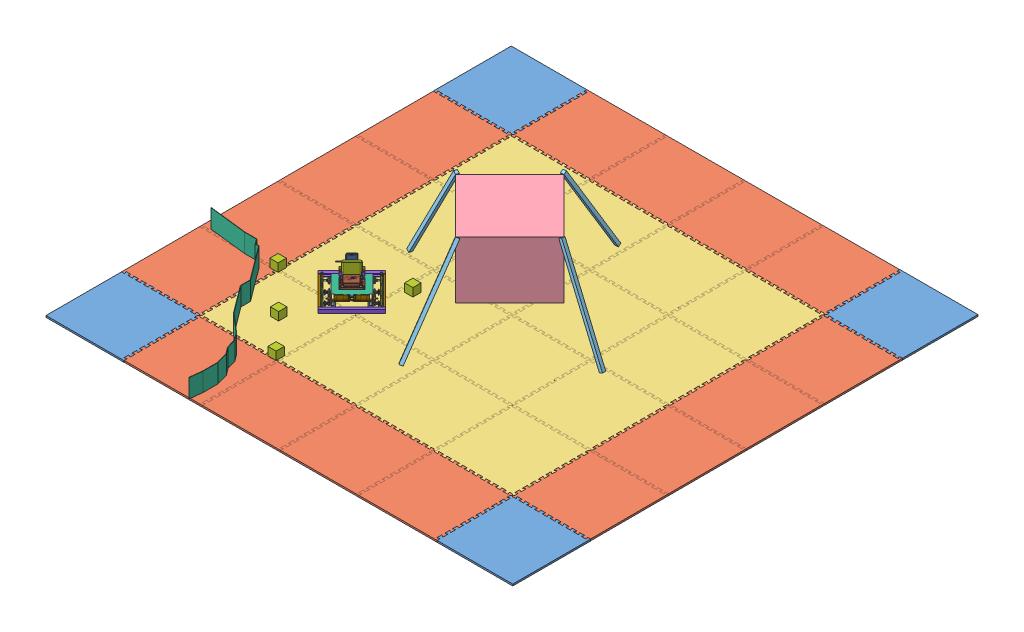
SolidWorks assembly FIELD_RelicRecovery_Perimeter and Tiles, configuration Default. Lengths in mm.
Overall size (3603.71 799.92 3631.27).
152 component instances, 29 part files, 1 mates.
Components (placement in the parent):
- FIELD_RelicRecovery_Tile Field-1: FIELD_RelicRecovery_Tile Field [Default] at (-1733.8336 13.8557 1782.5499) size (3603.71 12.7 3603.65)
  - FIELD_RelicRecovery_Corner soft tile-1: FIELD_RelicRecovery_Corner soft tile [Default] at (291.8914 -12.7 -291.8914) size (602.83 12.7 602.83)
  - FIELD_RelicRecovery_Corner soft tile-2: FIELD_RelicRecovery_Corner soft tile [Default] at (3306.0551 -12.7 -297.6546) x (0 0 -1) z (1 0 0) size (602.83 12.7 602.83)
  - FIELD_RelicRecovery_Corner soft tile-3: FIELD_RelicRecovery_Corner soft tile [Default] at (286.1281 -12.7 -3306.0551) x (0 0 1) z (-1 0 0) size (602.83 12.7 602.83)
  - FIELD_RelicRecovery_Corner soft tile-4: FIELD_RelicRecovery_Corner soft tile [Default] at (3300.2918 -12.7 -3311.7596) x (-1 0 0) z (0 0 -1) size (602.83 12.7 602.83)
  - FIELD_RelicRecovery_Side soft tile-1: FIELD_RelicRecovery_Side soft tile [Default] at (894.7241 -12.7 -293.0469) size (621.88 12.7 602.83)
  - FIELD_RelicRecovery_Side soft tile-2: FIELD_RelicRecovery_Side soft tile [Default] at (290.7358 -12.7 -894.7241) x (0 0 1) z (-1 0 0) size (621.88 12.7 602.83)
  - FIELD_RelicRecovery_Side soft tile-3: FIELD_RelicRecovery_Side soft tile [Default] at (1497.5568 -12.7 -294.2025) size (621.88 12.7 602.83)
  - FIELD_RelicRecovery_Side soft tile-4: FIELD_RelicRecovery_Side soft tile [Default] at (2100.3896 -12.7 -295.3581) size (621.88 12.7 602.83)
  - FIELD_RelicRecovery_Side soft tile-5: FIELD_RelicRecovery_Side soft tile [Default] at (2703.2223 -12.7 -296.5137) size (621.88 12.7 602.83)
  - FIELD_RelicRecovery_Side soft tile-6: FIELD_RelicRecovery_Side soft tile [Default] at (289.5802 -12.7 -1497.5568) x (0 0 1) z (-1 0 0) size (621.88 12.7 602.83)
  - FIELD_RelicRecovery_Side soft tile-7: FIELD_RelicRecovery_Side soft tile [Default] at (288.4246 -12.7 -2100.3896) x (0 0 1) z (-1 0 0) size (621.88 12.7 602.83)
  - FIELD_RelicRecovery_Side soft tile-8: FIELD_RelicRecovery_Side soft tile [Default] at (287.2691 -12.7 -2703.2223) x (0 0 1) z (-1 0 0) size (621.88 12.7 602.83)
  - FIELD_RelicRecovery_Side soft tile-9: FIELD_RelicRecovery_Side soft tile [Default] at (888.9609 -12.7 -3307.196) x (-1 0 0) z (0 0 -1) size (621.88 12.7 602.83)
  - FIELD_RelicRecovery_Side soft tile-10: FIELD_RelicRecovery_Side soft tile [Default] at (1491.7936 -12.7 -3308.3369) x (-1 0 0) z (0 0 -1) size (621.88 12.7 602.83)
  - FIELD_RelicRecovery_Side soft tile-11: FIELD_RelicRecovery_Side soft tile [Default] at (2094.6264 -12.7 -3309.4778) x (-1 0 0) z (0 0 -1) size (621.88 12.7 602.83)
  - FIELD_RelicRecovery_Side soft tile-12: FIELD_RelicRecovery_Side soft tile [Default] at (2697.4591 -12.7 -3310.6187) x (-1 0 0) z (0 0 -1) size (621.88 12.7 602.83)
  - FIELD_RelicRecovery_Side soft tile-13: FIELD_RelicRecovery_Side soft tile [Default] at (3301.4327 -12.7 -2708.9269) x (0 0 -1) z (1 0 0) size (621.88 12.7 602.83)
  - FIELD_RelicRecovery_Side soft tile-14: FIELD_RelicRecovery_Side soft tile [Default] at (3302.5737 -12.7 -2106.0942) x (0 0 -1) z (1 0 0) size (621.88 12.7 602.83)
  - FIELD_RelicRecovery_Side soft tile-15: FIELD_RelicRecovery_Side soft tile [Default] at (3303.7146 -12.7 -1503.2614) x (0 0 -1) z (1 0 0) size (621.88 12.7 602.83)
  - FIELD_RelicRecovery_Side soft tile-16: FIELD_RelicRecovery_Side soft tile [Default] at (3304.8555 -12.7 -900.4287) x (0 0 -1) z (1 0 0) size (621.88 12.7 602.83)
  - FIELD_RelicRecovery_Standard soft tile-1: FIELD_RelicRecovery_Standard soft tile [Default] at (893.5685 -12.7 -895.8797) size (621.88 12.7 621.88)
  - FIELD_RelicRecovery_Standard soft tile-2: FIELD_RelicRecovery_Standard soft tile [Default] at (892.413 -12.7 -1498.7124) size (621.88 12.7 621.88)
  - FIELD_RelicRecovery_Standard soft tile-3: FIELD_RelicRecovery_Standard soft tile [Default] at (891.2574 -12.7 -2101.5452) size (621.88 12.7 621.88)
  - FIELD_RelicRecovery_Standard soft tile-4: FIELD_RelicRecovery_Standard soft tile [Default] at (890.1018 -12.7 -2704.3779) size (621.88 12.7 621.88)
  - FIELD_RelicRecovery_Standard soft tile-5: FIELD_RelicRecovery_Standard soft tile [Default] at (1496.4013 -12.7 -897.0353) size (621.88 12.7 621.88)
  - FIELD_RelicRecovery_Standard soft tile-6: FIELD_RelicRecovery_Standard soft tile [Default] at (1495.2457 -12.7 -1499.868) size (621.88 12.7 621.88)
  - FIELD_RelicRecovery_Standard soft tile-7: FIELD_RelicRecovery_Standard soft tile [Default] at (1494.0901 -12.7 -2102.7007) size (621.88 12.7 621.88)
  - FIELD_RelicRecovery_Standard soft tile-8: FIELD_RelicRecovery_Standard soft tile [Default] at (1492.9345 -12.7 -2705.5335) size (621.88 12.7 621.88)
  - FIELD_RelicRecovery_Standard soft tile-9: FIELD_RelicRecovery_Standard soft tile [Default] at (2099.234 -12.7 -898.1908) size (621.88 12.7 621.88)
  - FIELD_RelicRecovery_Standard soft tile-10: FIELD_RelicRecovery_Standard soft tile [Default] at (2098.0784 -12.7 -1501.0236) size (621.88 12.7 621.88)
  - FIELD_RelicRecovery_Standard soft tile-11: FIELD_RelicRecovery_Standard soft tile [Default] at (2096.9228 -12.7 -2103.8563) size (621.88 12.7 621.88)
  - FIELD_RelicRecovery_Standard soft tile-12: FIELD_RelicRecovery_Standard soft tile [Default] at (2095.7673 -12.7 -2706.689) size (621.88 12.7 621.88)
  - FIELD_RelicRecovery_Standard soft tile-13: FIELD_RelicRecovery_Standard soft tile [Default] at (2702.0667 -12.7 -899.3464) size (621.88 12.7 621.88)
  - FIELD_RelicRecovery_Standard soft tile-14: FIELD_RelicRecovery_Standard soft tile [Default] at (2700.9112 -12.7 -1502.1791) size (621.88 12.7 621.88)
  - FIELD_RelicRecovery_Standard soft tile-15: FIELD_RelicRecovery_Standard soft tile [Default] at (2699.7556 -12.7 -2105.0119) size (621.88 12.7 621.88)
  - FIELD_RelicRecovery_Standard soft tile-16: FIELD_RelicRecovery_Standard soft tile [Default] at (2698.6 -12.7 -2707.8446) size (621.88 12.7 621.88)
- Assem1-1: Assem1 [Default] at (-345.7098 170.5102 -63.598) x (0.707107 0 -0.707107) z (0.707107 0 0.707107) size (1212.6 747.66 1171.24)
  - landerBody-1: landerBody [Default] at (321.6828 178.1754 363.226) size (591.82 439.42 591.82)
  - landerLegs-1: landerLegs [Default] at (757.5041 -108.5653 925.7867) x (-0.665044 -0.418518 -0.618514) z (0.692784 -0.036473 -0.720222) size (25.4 797.56 25.4)
  - landerLegs-2: landerLegs [Default] at (833.0645 -63.9982 -208.5204) x (0.534547 0.510671 -0.673406) z (0.758575 0.061365 0.64869) size (25.4 797.56 25.4)
  - landerLegs-3: landerLegs [Default] at (-342.3782 -98.5367 874.384) x (-0.919891 0.356278 -0.163912) z (0.051837 -0.303829 -0.951315) size (25.4 797.56 25.4)
  - landerLegs-4: landerLegs [Default] at (-306.2525 -82.7813 -199.247) x (0.456169 -0.450226 0.767598) z (-0.830357 0.094851 0.5491) size (25.4 797.56 25.4)
- crter lol-1: crter lol [Default] at (-875.4653 178.5063 970.4536) size (1061.15 143 1222.76)
- gold-1: gold [Default] at (-1161.7992 41.3904 615.4522) size (63.5 63.5 63.5)
- gold-2: gold [Default] at (-861.9809 13.8557 911.0218) size (63.5 63.5 63.5)
- gold-3: gold [Default] at (-582.5643 38.5098 1209.8894) size (63.5 63.5 63.5)
- CH_ASSEM_FULL-2: CH_ASSEM_FULL [Default] at (-816.9923 -21.3569 484.7087) x (0.707107 0 -0.707107) z (0.707107 0 0.707107) size (404.11 208.98 368.3)
  - CH_ASSEM_Base-1: CH_ASSEM_Base [Default] at (-90.7761 -10.2499 -116.5851) size (368.3 25.4 368.3)
    - CH_FrontBackChannel-2: CH_FrontBackChannel [Default] at (378.7562 204.4057 248.334) x (0 1 0) z (0 0 1) size (25.4 368.3 25.4)
    - CH_SideOuterChannel-2: CH_SideOuterChannel [Default] at (23.1562 207.5807 226.109) x (0 1 0) z (1 0 0) size (19.05 361.95 12.7)
    - CH_FrontBackChannel-3: CH_FrontBackChannel [Default] at (378.7562 229.8057 565.834) x (0 -1 0) z (0 0 -1) size (25.4 368.3 25.4)
    - CH_SideInnerChannel-3: CH_SideInnerChannel [Default] at (80.0522 207.5807 588.059) x (0 1 0) z (-1 0 0) size (19.05 361.95 25.4)
    - CH_SideInnerChannel-4: CH_SideInnerChannel [Default] at (309.1602 226.6307 588.059) x (0 -1 0) z (1 0 0) size (19.05 361.95 25.4)
    - CH_SideOuterChannel-5: CH_SideOuterChannel [Default] at (366.0562 226.6307 226.109) x (0 -1 0) z (-1 0 0) size (19.05 361.95 12.7)
  - CH_ASSEM_DriveWheel-1: CH_ASSEM_DriveWheel [Default] at (59.5626 215.0895 411.9658) x (0 0 1) z (-1 0 0) size (123.02 123.02 97.03)
    - CH_ASSEM_BearingBlock-1: CH_ASSEM_BearingBlock [Default] at (2.3581 -14.5837 48.57) size (29.51 14.04 11.53)
      - PART_BearingBlock-1: PART_BearingBlock [Default] at (-29.5139 0 12.1915) x (1 0 0) z (0 -1 0) size (29.51 9.53 12.7)
      - PART_BearingThroughBoreLong-1: PART_BearingThroughBoreLong [Default] at (-14.7569 7.5406 21.7165) size (13 13 11)
    - CH_ASSEM_DriveWheelShaft-1: CH_ASSEM_DriveWheelShaft [Default] at (-19.3547 -19.6717 70.3125) x (0.866025 -0.5 0) z (0 0 1) size (90.05 90.05 96.5)
      - PART_Gear30Tooth-1: PART_Gear30Tooth [Default] at (-0.2904 14.4147 9.474) size (24.32 24.24 15)
      - PART_HexShaft75mm-1: PART_HexShaft75mm [Default] at (-0.2904 14.4147 -9.026) size (5 5.77 75)
      - PART_Sprocket15Tooth-1: PART_Sprocket15Tooth [Default] at (-0.2904 14.4147 32.474) size (33.59 33.42 15)
      - PART_TractionWheel90mm-1: PART_TractionWheel90mm [Default] at (-0.2904 14.4147 47.474) size (90.05 90.05 80)
      - PART_ShaftCollar-1: PART_ShaftCollar [Default] at (-0.2904 14.4147 20.974) size (13 13 8)
    - CH_ASSEM_BearingBlock-2: CH_ASSEM_BearingBlock [Default] at (-27.1558 -14.5837 149.0031) x (-1 0 0) z (0 0 -1) size (29.51 14.04 11.53)
      - PART_BearingBlock-1: PART_BearingBlock [Default] at (-29.5139 0 12.1915) x (1 0 0) z (0 -1 0) size (29.51 9.53 12.7)
      - PART_BearingThroughBoreLong-1: PART_BearingThroughBoreLong [Default] at (-14.7569 7.5406 21.7165) size (13 13 11)
  - PART_ASSEM_MotorHDHexRotating-1: PART_ASSEM_MotorHDHexRotating [Default] at (134.2476 254.6096 293.9221) x (0 -0.92311 0.384536) z (-1 0 0) size (38 39.44 154.16)
    - PART_MotorHDHex_Shell-1: PART_MotorHDHex_Shell [Default] at (52.6409 85.4657 114.2715) size (38 39.44 128.25)
    - PART_MotorHDHex_RotatingHex-1: PART_MotorHDHex_RotatingHex [Default] at (52.6787 94.995 172.8795) x (0.858442 -0.512911 0) z (0.512911 0.858442 0) size (5.06 33.53 5.84)
  - PART_Gear60Tooth-1: PART_Gear60Tooth [Default] at (-20.2239 241.5359 399.567) x (0 0.989669 0.143372) z (1 0 0) size (47.04 47.04 15)
  - PART_MotorMount-1: PART_MotorMount [Default] at (6.2756 238.7668 404.1993) x (0 0 -1) z (1 0 0) size (72 44.98 12.7)
  - CH_Assem_CentreWheel-1: CH_Assem_CentreWheel [Default] at (2.6857 228.0574 315.7728) x (0 0 -1) z (-1 0 0) size (123.02 123.02 97.03)
    - CH_ASSEM_BearingBlock-1: CH_ASSEM_BearingBlock [Default] at (40.0308 14.8515 -8.3069) size (29.51 14.04 11.53)
      - PART_BearingBlock-1: PART_BearingBlock [Default] at (-29.5139 0 12.1915) x (1 0 0) z (0 -1 0) size (29.51 9.53 12.7)
      - PART_BearingThroughBoreLong-1: PART_BearingThroughBoreLong [Default] at (-14.7569 7.5406 21.7165) size (13 13 11)
    - CH_Assem_CentreWheelShaft-1: CH_Assem_CentreWheelShaft [Default] at (67.892 -5.5775 97.812) x (-0.866025 -0.5 0) z (0 0 -1) size (90.05 90.05 96.5)
      - PART_HexShaft75mm-1: PART_HexShaft75mm [Default] at (22.9236 45.5315 18.4024) size (5 5.77 75)
      - PART_Sprocket15Tooth-1: PART_Sprocket15Tooth [Default] at (22.9236 45.5315 51.9024) size (33.59 33.42 15)
      - PART_Sprocket20Tooth-1: PART_Sprocket20Tooth [Default] at (22.9236 45.5315 74.9024) size (43.5 43.5 15)
      - PART_TractionWheel90mm-1: PART_TractionWheel90mm [Default] at (22.9236 45.5315 36.9024) size (90.05 90.05 80)
      - PART_ShaftCollar-1: PART_ShaftCollar [Default] at (22.9236 45.5315 63.4024) size (13 13 8)
    - CH_ASSEM_BearingBlock-2: CH_ASSEM_BearingBlock [Default] at (10.5169 14.8515 92.1262) x (-1 0 0) z (0 0 -1) size (29.51 14.04 11.53)
      - PART_BearingBlock-1: PART_BearingBlock [Default] at (-29.5139 0 12.1915) x (1 0 0) z (0 -1 0) size (29.51 9.53 12.7)
      - PART_BearingThroughBoreLong-1: PART_BearingThroughBoreLong [Default] at (-14.7569 7.5406 21.7165) size (13 13 11)
  - CH_ASSEM_EndWheel-1: CH_ASSEM_EndWheel [Default] at (-69.5235 200.5058 196.1878) x (0 0 1) z (-1 0 0) size (123.02 123.02 97.03)
    - CH_ASSEM_BearingBlock-1: CH_ASSEM_BearingBlock [Default] at (0 0 -80.5161) size (29.51 14.04 11.53)
      - PART_BearingBlock-1: PART_BearingBlock [Default] at (-29.5139 0 12.1915) x (1 0 0) z (0 -1 0) size (29.51 9.53 12.7)
      - PART_BearingThroughBoreLong-1: PART_BearingThroughBoreLong [Default] at (-14.7569 7.5406 21.7165) size (13 13 11)
    - CH_ASSEM_EndWheelShaft-1: CH_ASSEM_EndWheelShaft [Default] at (-15.9553 -39.3245 28.8345) x (-0.866025 0.5 0) z (0 0 -1) size (90.05 90.05 96.5)
      - PART_HexShaft75mm-1: PART_HexShaft75mm [Default] at (22.3948 41.1855 21.634) size (5 5.77 75)
      - PART_Spacer15mm-1: PART_Spacer15mm [Default] at (22.3948 41.1855 55.134) size (8.79 8.79 15)
      - PART_Sprocket20Tooth-1: PART_Sprocket20Tooth [Default] at (22.3948 41.1855 78.134) size (43.5 43.5 15)
      - PART_TractionWheel90mm-1: PART_TractionWheel90mm [Default] at (22.3948 41.1855 40.134) size (90.05 90.05 80)
      - PART_ShaftCollar-1: PART_ShaftCollar [Default] at (22.3948 41.1855 66.634) size (13 13 8)
    - CH_ASSEM_BearingBlock-2: CH_ASSEM_BearingBlock [Default] at (-29.5139 0 19.917) x (-1 0 0) z (0 0 -1) size (29.51 14.04 11.53)
      - PART_BearingBlock-1: PART_BearingBlock [Default] at (-29.5139 0 12.1915) x (1 0 0) z (0 -1 0) size (29.51 9.53 12.7)
      - PART_BearingThroughBoreLong-1: PART_BearingThroughBoreLong [Default] at (-14.7569 7.5406 21.7165) size (13 13 11)
  - PART_ASSEM_MotorHDHexRotating-2: PART_ASSEM_MotorHDHexRotating [Default] at (73.4126 157.4229 334.4067) x (0 0.92311 -0.384536) z (1 0 0) size (38 39.44 154.16)
    - PART_MotorHDHex_Shell-1: PART_MotorHDHex_Shell [Default] at (52.6409 85.4657 114.2715) size (38 39.44 128.25)
    - PART_MotorHDHex_RotatingHex-1: PART_MotorHDHex_RotatingHex [Default] at (52.6787 94.995 172.8795) x (0.858442 -0.512911 0) z (0.512911 0.858442 0) size (5.06 33.53 5.84)
  - CH_ASSEM_DriveWheel-2: CH_ASSEM_DriveWheel [Default] at (148.0976 215.0895 387.1681) x (0 0 -1) z (1 0 0) size (123.02 123.02 97.03)
    - CH_ASSEM_BearingBlock-1: CH_ASSEM_BearingBlock [Default] at (2.3581 -14.5837 48.57) size (29.51 14.04 11.53)
      - PART_BearingBlock-1: PART_BearingBlock [Default] at (-29.5139 0 12.1915) x (1 0 0) z (0 -1 0) size (29.51 9.53 12.7)
      - PART_BearingThroughBoreLong-1: PART_BearingThroughBoreLong [Default] at (-14.7569 7.5406 21.7165) size (13 13 11)
    - CH_ASSEM_DriveWheelShaft-1: CH_ASSEM_DriveWheelShaft [Default] at (-19.3547 -19.6717 70.3125) x (0.866025 -0.5 0) z (0 0 1) size (90.05 90.05 96.5)
      - PART_Gear30Tooth-1: PART_Gear30Tooth [Default] at (-0.2904 14.4147 9.474) size (24.32 24.24 15)
      - PART_HexShaft75mm-1: PART_HexShaft75mm [Default] at (-0.2904 14.4147 -9.026) size (5 5.77 75)
      - PART_Sprocket15Tooth-1: PART_Sprocket15Tooth [Default] at (-0.2904 14.4147 32.474) size (33.59 33.42 15)
      - PART_TractionWheel90mm-1: PART_TractionWheel90mm [Default] at (-0.2904 14.4147 47.474) size (90.05 90.05 80)
      - PART_ShaftCollar-1: PART_ShaftCollar [Default] at (-0.2904 14.4147 20.974) size (13 13 8)
    - CH_ASSEM_BearingBlock-2: CH_ASSEM_BearingBlock [Default] at (-27.1558 -14.5837 149.0031) x (-1 0 0) z (0 0 -1) size (29.51 14.04 11.53)
      - PART_BearingBlock-1: PART_BearingBlock [Default] at (-29.5139 0 12.1915) x (1 0 0) z (0 -1 0) size (29.51 9.53 12.7)
      - PART_BearingThroughBoreLong-1: PART_BearingThroughBoreLong [Default] at (-14.7569 7.5406 21.7165) size (13 13 11)
  - PART_Gear60Tooth-2: PART_Gear60Tooth [Default] at (227.8841 241.5359 399.567) x (0 -0.989669 -0.143372) z (-1 0 0) size (47.04 47.04 15)
  - PART_MotorMount-2: PART_MotorMount [Default] at (213.2836 238.7668 404.1993) x (0 0 -1) z (1 0 0) size (72 44.98 12.7)
  - CH_Assem_CentreWheel-2: CH_Assem_CentreWheel [Default] at (204.9745 228.0574 265.2251) x (0 0 1) z (1 0 0) size (123.02 123.02 97.03)
    - CH_ASSEM_BearingBlock-1: CH_ASSEM_BearingBlock [Default] at (40.0308 14.8515 -8.3069) size (29.51 14.04 11.53)
      - PART_BearingBlock-1: PART_BearingBlock [Default] at (-29.5139 0 12.1915) x (1 0 0) z (0 -1 0) size (29.51 9.53 12.7)
      - PART_BearingThroughBoreLong-1: PART_BearingThroughBoreLong [Default] at (-14.7569 7.5406 21.7165) size (13 13 11)
    - CH_Assem_CentreWheelShaft-1: CH_Assem_CentreWheelShaft [Default] at (67.892 -5.5775 97.812) x (-0.866025 -0.5 0) z (0 0 -1) size (90.05 90.05 96.5)
      - PART_HexShaft75mm-1: PART_HexShaft75mm [Default] at (22.9236 45.5315 18.4024) size (5 5.77 75)
      - PART_Sprocket15Tooth-1: PART_Sprocket15Tooth [Default] at (22.9236 45.5315 51.9024) size (33.59 33.42 15)
      - PART_Sprocket20Tooth-1: PART_Sprocket20Tooth [Default] at (22.9236 45.5315 74.9024) size (43.5 43.5 15)
      - PART_TractionWheel90mm-1: PART_TractionWheel90mm [Default] at (22.9236 45.5315 36.9024) size (90.05 90.05 80)
      - PART_ShaftCollar-1: PART_ShaftCollar [Default] at (22.9236 45.5315 63.4024) size (13 13 8)
    - CH_ASSEM_BearingBlock-2: CH_ASSEM_BearingBlock [Default] at (10.5169 14.8515 92.1262) x (-1 0 0) z (0 0 -1) size (29.51 14.04 11.53)
      - PART_BearingBlock-1: PART_BearingBlock [Default] at (-29.5139 0 12.1915) x (1 0 0) z (0 -1 0) size (29.51 9.53 12.7)
      - PART_BearingThroughBoreLong-1: PART_BearingThroughBoreLong [Default] at (-14.7569 7.5406 21.7165) size (13 13 11)
  - CH_ASSEM_EndWheel-2: CH_ASSEM_EndWheel [Default] at (277.1837 215.5871 196.1878) x (0 0 1) z (1 0 0) size (123.02 123.02 97.03)
    - CH_ASSEM_BearingBlock-1: CH_ASSEM_BearingBlock [Default] at (0 0 -80.5161) size (29.51 14.04 11.53)
      - PART_BearingBlock-1: PART_BearingBlock [Default] at (-29.5139 0 12.1915) x (1 0 0) z (0 -1 0) size (29.51 9.53 12.7)
      - PART_BearingThroughBoreLong-1: PART_BearingThroughBoreLong [Default] at (-14.7569 7.5406 21.7165) size (13 13 11)
    - CH_ASSEM_EndWheelShaft-1: CH_ASSEM_EndWheelShaft [Default] at (-15.9553 -39.3245 28.8345) x (-0.866025 0.5 0) z (0 0 -1) size (90.05 90.05 96.5)
      - PART_HexShaft75mm-1: PART_HexShaft75mm [Default] at (22.3948 41.1855 21.634) size (5 5.77 75)
      - PART_Spacer15mm-1: PART_Spacer15mm [Default] at (22.3948 41.1855 55.134) size (8.79 8.79 15)
      - PART_Sprocket20Tooth-1: PART_Sprocket20Tooth [Default] at (22.3948 41.1855 78.134) size (43.5 43.5 15)
      - PART_TractionWheel90mm-1: PART_TractionWheel90mm [Default] at (22.3948 41.1855 40.134) size (90.05 90.05 80)
      - PART_ShaftCollar-1: PART_ShaftCollar [Default] at (22.3948 41.1855 66.634) size (13 13 8)
    - CH_ASSEM_BearingBlock-2: CH_ASSEM_BearingBlock [Default] at (-29.5139 0 19.917) x (-1 0 0) z (0 0 -1) size (29.51 14.04 11.53)
      - PART_BearingBlock-1: PART_BearingBlock [Default] at (-29.5139 0 12.1915) x (1 0 0) z (0 -1 0) size (29.51 9.53 12.7)
      - PART_BearingThroughBoreLong-1: PART_BearingThroughBoreLong [Default] at (-14.7569 7.5406 21.7165) size (13 13 11)
  - CH_BaseSheet-1: CH_BaseSheet [Default] at (-10.7239 216.3808 347.6489) size (229.11 3.17 215.9)
  - CH_ASSEM_BatteryPhone-1: CH_ASSEM_BatteryPhone [Default] at (39.7502 187.7674 170.7548) x (0 0 -1) z (1 0 0) size (44.45 133.58 161.51)
    - PART_BatterySlim12V-1: PART_BatterySlim12V [Default] at (26.3058 77.0384 64.08) x (0 -1 0) z (0 0 1) size (90.56 23.03 147.25)
    - PART_SlimBatteryClip-1: PART_SlimBatteryClip [Default] at (39.0058 31.7884 107.3076) x (0 0 -1) z (1 0 0) size (18.01 28.57 25.4)
    - PART_SlimBatteryClip-2: PART_SlimBatteryClip [Default] at (13.6058 31.7884 20.8523) x (0 0 1) z (-1 0 0) size (18.01 28.57 25.4)
    - PART_PhoneSupportSheet-1: PART_PhoneSupportSheet [Default] at (58.0558 60.3634 134.692) x (0 0 -1) z (1 0 0) size (141.22 3.17 44.45)
    - PART_ZTESpeed-1: PART_ZTESpeed [Default] at (40.0121 98.6181 70.154) x (0 0 1) z (-1 0 0) size (68.17 133.58 10.49)
  - PART_ExpansionHub-1: PART_ExpansionHub [Default] at (103.8301 219.4847 232.4629) x (0 0 1) z (-1 0 0) size (103 29.58 143)
- gold-4: gold [Default] at (-287.7382 229.9403 448.7105) size (63.5 63.5 63.5)
Mates (geometry in assembly coordinates):
- Coincident2: coincident anti-aligned: plane of FIELD_RelicRecovery_Tile Field-1/FIELD_RelicRecovery_Standard soft tile-1 through (-840.2651 13.8557 886.6702) normal (0 1 0); plane of gold-2 through (-861.9809 13.8557 911.0218) normal (0 -1 0)
